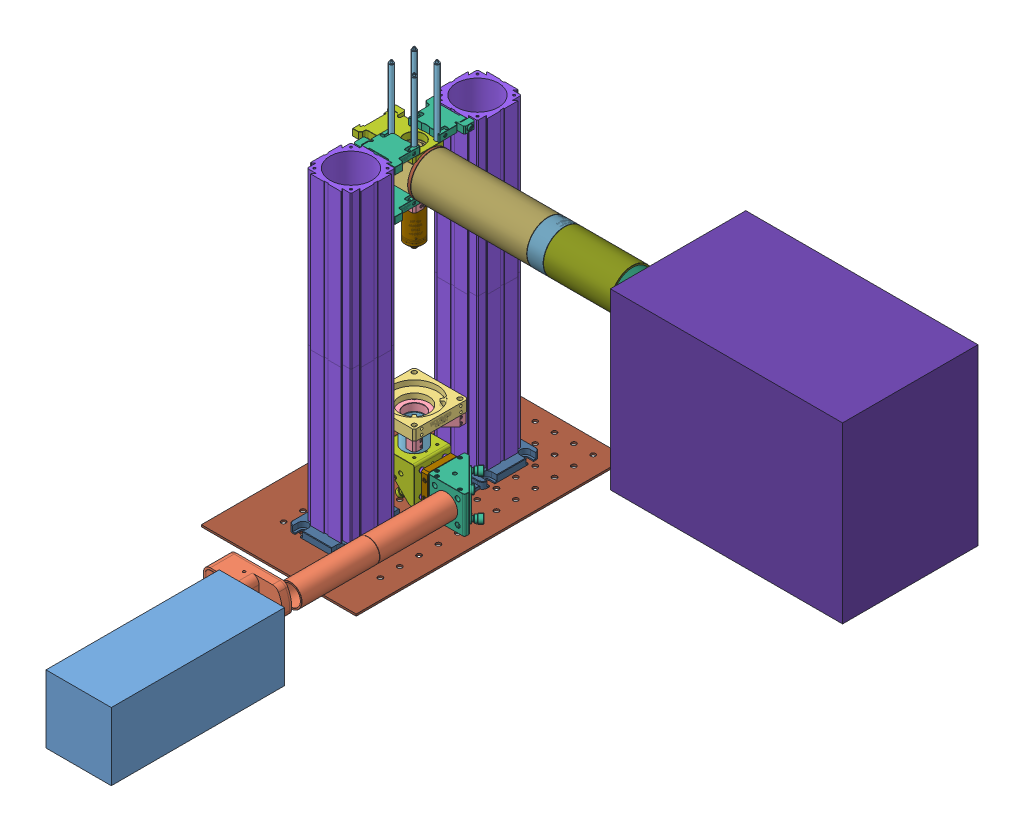
SolidWorks assembly Assembly, configuration Default. Lengths in mm.
Overall size (752.75 517.15 684.37).
51 component instances, 33 part files, 26 mates.
Components (placement in the parent):
- Laser-1: Laser [Default] at (-432.7153 -246.2224 392.8569) x (0 0 1) z (-1 0 0) size (238.02 88.9 85.74)
- SH05-Solidworks-1: SH05-Solidworks [Default] at (-478.4983 -151.3145 267.4556) x (0 1 0) z (0 0 -1) size (57.1 81.96 34.87)
- Objective Sub-Assembly-1: Objective Sub-Assembly [Default] at (-599.9053 226.5168 -25.2284) x (1 0 0) z (0 -1 0) size (97.86 248.79 490.2)
  - CM1-DCH-Solidworks-1: CM1-DCH-Solidworks [Web Assembly] at (101.1512 25.2284 74.1168) size (38.1 45.72 38.1)
  - CP16-Solidworks-1: CP16-Solidworks [Default] at (83.0447 27.4143 114.1512) size (41.22 40.64 8.89)
  - ER6-P4-Solidworks-1: ER6-P4-Solidworks [Default] at (115.9512 38.6905 31.8406) x (0.631657 -0.775248 0) z (-0.775248 -0.631657 0) size (5.99 157.48 5.99)
  - ER6-P4-Solidworks-2: ER6-P4-Solidworks [Default] at (114.7082 9.6603 31.8406) x (-0.373438 -0.927655 0) z (-0.927655 0.373438 0) size (5.99 157.48 5.99)
  - ER6-P4-Solidworks-3: ER6-P4-Solidworks [Default] at (85.1563 39.0388 31.8406) x (0.116187 -0.993227 0) z (-0.993227 -0.116187 0) size (5.99 157.48 5.99)
  - ER6-P4-Solidworks-4: ER6-P4-Solidworks [Default] at (87.3845 11.1687 36.8125) x (0.986967 -0.160923 0) z (0.160923 0.986967 0) size (5.99 157.48 5.99)
  - RCA2-Solidworks-1: RCA2-Solidworks [Default] at (87.6791 34.1856 4.2312) size (56.73 41.06 8.89)
  - RCA2-Solidworks-2: RCA2-Solidworks [Default] at (114.6233 16.2713 4.2312) x (-1 0 0) z (0 0 1) size (56.73 41.06 8.89)
  - RCA1-Solidworks-1: RCA1-Solidworks [Default] at (125.4438 -3.2318 -2.9001) x (0 1 0) z (0 0 1) size (56.5 73.55 8.89)
  - XT66-200-Solidworks-1: XT66-200-Solidworks [Default] at origin size (66.04 66.04 200)
  - XT66-200-Solidworks-2: XT66-200-Solidworks [Default] at (0 -166.04 0) size (66.04 66.04 200)
  - N40X-NIR-Solidworks-1: N40X-NIR-Solidworks [Default] at (101.1512 25.2284 137.1966) x (0 0 1) z (-0.615109 0.788442 0) size (61.98 27.94 27.94)
  - RCA2-Solidworks-3: RCA2-Solidworks [Default] at (114.6233 16.2713 60.4974) x (-1 0 0) z (0 0 1) size (56.73 41.06 8.89)
  - RCA2-Solidworks-4: RCA2-Solidworks [Default] at (87.6791 34.1856 60.4974) size (56.73 41.06 8.89)
  - XT66-200-Solidworks-3: XT66-200-Solidworks [Default] at (0 0 199.9996) size (66.04 66.04 200)
  - XT66-200-Solidworks-4: XT66-200-Solidworks [Default] at (0 -166.04 199.9996) size (66.04 66.04 200)
  - XT66P1-Solidworks-1: XT66P1-Solidworks [Default] at (101.1512 108.2611 445.7898) x (1 0 0) z (0 1 0) size (76.2 8.89 89.28)
  - XT66P1-Solidworks-2: XT66P1-Solidworks [Default] at (101.1385 -57.7916 445.7898) x (0 1 0) z (-1 0 0) size (76.2 8.89 89.28)
- Tank Sub-Assembly-1: Tank Sub-Assembly [Default] at origin size (492.39 222.91 245.75) (hidden)
  - WaterBath-1: WaterBath [Default] at (-614.8457 -4.3008 0) size (203.2 101.6 101.6)
  - L490-Solidworks-1: L490-Solidworks [Default] at (-624.5838 -100.8719 -9.0343) x (0 0 -1) z (1 0 0) size (245.75 83.31 101.6)
  - LX20-Solidworks-1: LX20-Solidworks [Chamfers] at (-650.9996 -116.3058 97.2581) size (132.4 38.28 116.16)
  - Opticell-1: Opticell [Default] at (-256.3578 52.6159 0) x (0.739747 0.672885 0) z (0 0 1) size (76.36 12.75 129.72)
- Camera Sub-Assembly-1: Camera Sub-Assembly [Default] at (-482.498 152.4 0) x (0 0.641515 0.767111) z (-1 0 0) size (71.93 71.93 328.57)
  - SM1A2-Solidworks-1: SM1A2-Solidworks [Default] at (0 0 -2.794) size (55.88 55.88 7.37)
  - SM2E60-Solidworks-1: SM2E60-Solidworks [Default] at (0 0 -83.312) x (-1 0 0) z (0 0 -1) size (55.88 55.88 155.45)
  - SM2NFM2-Solidworks-1: SM2NFM2-Solidworks [Default] at (0 0 -316.9027) x (0 1 0) z (-1 0 0) size (63.5 16.37 63.5)
  - TTL200-S8-Solidworks-1: TTL200-S8-Solidworks [Default] at (0 0 -170.337) size (55.88 55.88 28)
  - SM2V15-Solidworks-1: SM2V15-Solidworks [Default] at (18.0496 -29.8565 -319.6416) x (0 0 -1) z (0.951776 0.306793 0) size (51.56 57.15 57.15)
  - SM2M35-Solidworks-1: SM2M35-Solidworks [Default] at (-13.4416 4.8034 -237.3095) x (0.972414 0.233264 0) z (0 0 1) size (55.88 55.88 88.9)
- hpvx2-1: hpvx2 [Default] at origin size (311.15 228.6 177.8)
- Small Condenser Adjustable Sub-Assembly-1: Small Condenser Adjustable Sub-Assembly [Default] at (-430.8557 -214.193 -104.0018) x (0 -1 0) z (1 0 0) size (105.41 276.48 128.6)
  - LB1437-Solidworks-1: LB1437-Solidworks [Default] at (-24.13 -280.0439 -1.8596) x (0.911373 0 -0.411581) z (0 -1 0) size (25.4 25.4 3.05)
  - LB1761-Solidworks-1: LB1761-Solidworks [Default] at (-24.13 -135.2439 -1.8596) x (0.962182 0 -0.272406) z (0 -1 0) size (25.4 25.4 8.98)
  - SM1L40-Solidworks-1: SM1L40-Solidworks [Default] at (-22.2262 -175.3632 -3.9514) x (-1 0 0) z (0 1 0) size (30.48 30.48 105.41)
  - SM1L40-Solidworks-2: SM1L40-Solidworks [Default] at (-22.2262 -277.7252 -3.9514) x (-1 0 0) z (0 1 0) size (30.48 30.48 105.41)
  - CSA1003-Solidworks-1: CSA1003-Solidworks [Default] at (-52.7119 -190.8909 -81.6147) x (0 -1 0) z (0 0 1) size (71.12 13.97 71.12)
  - LCP02-Solidworks-1: LCP02-Solidworks [Default] at (-80.01 -104.0019 -67.8996) x (0 0 -1) z (1 0 0) size (70.75 70.61 12.7)
  - SM1S10-Solidworks-1: SM1S10-Solidworks [Default] at (-60.96 -104.0019 -67.8996) x (1 0 0) z (0 -0.505002 0.863118) size (31.5 30.48 30.48)
  - KCB1C-Solidworks-1: KCB1C-Solidworks [Default] at (-24.13 -104.0019 -1.8596) x (0 0 -1) z (0 -1 0) size (51.13 48.49 51.11)
  - KCB1-Solidworks-1: KCB1-Solidworks [Default] at (0 -79.8719 -92.0296) x (-1 0 0) z (0 0 1) size (51.13 48.26 51.1)
  - ER1-Solidworks-1: ER1-Solidworks [Default] at (-9.7751 -90.4123 -33.5555) x (0.374639 -0.927171 0) z (-0.927171 -0.374639 0) size (5.99 30.48 5.99)
  - ER1-Solidworks-2: ER1-Solidworks [Default] at (-9.1095 -120.5526 -33.5555) x (0.735372 -0.677663 0) z (-0.677663 -0.735372 0) size (5.99 30.48 5.99)
  - ER1-Solidworks-3: ER1-Solidworks [Default] at (-40.6715 -89.1711 -33.5555) x (-0.604001 -0.796983 0) z (-0.796983 0.604001 0) size (5.99 30.48 5.99)
  - ER1-Solidworks-4: ER1-Solidworks [Default] at (-40.6266 -118.5953 -33.5555) x (-0.853706 -0.520755 0) z (-0.520755 0.853706 0) size (5.99 30.48 5.99)
  - CP08-Solidworks-1: CP08-Solidworks [Default] at (-24.13 -104.002 -34.2446) x (0 1 0) z (0 0 1) size (41.5 40.64 8.89)
  - CPB1-Solidworks-1: CPB1-Solidworks [Default] at (5.08 -151.627 -27.2596) x (0 -1 0) z (0 0 -1) size (95.25 10.79 15.24)
- Table-1: Table [Default] at (-498.7541 -221.559 0) x (0 0 1) z (-1 0 0) size (355.6 2.54 203.2)
Mates (geometry in assembly coordinates):
- Concentric1: concentric anti-aligned: circle of Laser-1; circle of SH05-Solidworks-1
- Parallel1: parallel aligned: plane of Laser-1 through (-475.5856 -157.3224 279.1461) normal (-1 0 0); plane of SH05-Solidworks-1 through (-500.0253 -206.573 244.0941) normal (-1 0 0)
- Parallel2: parallel aligned: plane of Laser-1 through (0 -151.1382 0) normal (0 -1 0); plane of ? through (-543.2054 -139.4288 -36.195) normal (0 -1 0)
- Parallel3: parallel aligned: plane of Laser-1; plane of ? through (-458.1154 -135.6188 -46.99) normal (0 0 -1)
- Concentric2: concentric aligned: circle of SH05-Solidworks-1; circle of ?
- Parallel4: parallel aligned: plane of Laser-1 through (-432.7153 -246.2224 392.8569) normal (0 -1 0); plane of Objective Sub-Assembly-1/XT66-200-Solidworks-2 through (-469.6457 -10.3834 -100.4861) normal (0 -1 0)
- Concentric3: concentric anti-aligned: circle of ?; circle of Objective Sub-Assembly-1/RCA1-Solidworks-1
- Concentric4: concentric anti-aligned: circle of Objective Sub-Assembly-1/CM1-DCH-Solidworks-1; circle of Camera Sub-Assembly-1/SM1A2-Solidworks-1
- Coincident9: coincident anti-aligned: plane of Objective Sub-Assembly-1/CM1-DCH-Solidworks-1 through (-479.704 133.35 19.05) normal (1 0 0); plane of Camera Sub-Assembly-1/SM1A2-Solidworks-1 through (-479.704 173.8331 -17.9239) normal (-1 0 0)
- Concentric5: concentric anti-aligned: cylinder of Camera Sub-Assembly-1/SM2M35-Solidworks-1 through (-254.346 152.4 0) axis (-1 0 0) radius 27.94; cylinder of hpvx2-1 through (-152.4 152.4 0) axis (1 0 0) radius 29.1375
- Parallel9: parallel aligned: plane of Laser-1 through (-432.7153 -157.3224 392.8569) normal (0 1 0); plane of hpvx2-1 through (0 228.6 0) normal (0 1 0)
- Coincident10: coincident anti-aligned: plane of Camera Sub-Assembly-1/SM2NFM2-Solidworks-1 through (-158.75 152.4547 -0.0457) normal (1 0 0); plane of hpvx2-1 through (-158.75 152.4 0) normal (-1 0 0)
- Coincident13: coordinate: point of hpvx2-1; point of assembly
- Parallel10: parallel anti-aligned: plane of hpvx2-1 through (0 228.6 0) normal (0 1 0); plane of Small Condenser Adjustable Sub-Assembly-1/CPB1-Solidworks-1 through (-473.3553 -219.019 -28.5749) normal (0 -1 0)
- Parallel11: parallel aligned: plane of hpvx2-1 through (152.4 228.6 88.9) normal (1 0 0); plane of Small Condenser Adjustable Sub-Assembly-1/CSA1003-Solidworks-1 through (-463.1954 -113.863 -35.56) normal (1 0 0)
- Concentric6: concentric anti-aligned: circle of Objective Sub-Assembly-1/RCA1-Solidworks-1; circle of Small Condenser Adjustable Sub-Assembly-1/CSA1003-Solidworks-1
- Concentric7: concentric anti-aligned: circle of Laser-1; circle of Small Condenser Adjustable Sub-Assembly-1/SM1L40-Solidworks-2
- Distance5: distance = 25.4 mm anti-aligned: plane of SH05-Solidworks-1 through (-462.8502 -190.2676 253.7461) normal (0 0 1); plane of Laser-1 through (-475.5856 -157.3224 279.1461) normal (0 0 -1)
- Distance6: distance = 12.7 mm anti-aligned: plane of SH05-Solidworks-1 through (-462.8502 -190.2676 241.5541) normal (0 0 -1); plane of Small Condenser Adjustable Sub-Assembly-1/SM1L40-Solidworks-2 through (-417.7293 -190.063 228.8541) normal (0 0 1)
- Parallel12: parallel anti-aligned: plane of hpvx2-1 through (152.4 228.6 88.9) normal (1 0 0); plane of Table-1 through (-600.3541 -219.019 -177.8) normal (-1 0 0)
- Coincident19: coincident aligned: plane of Table-1 through (-498.7541 -221.559 0) normal (0 0 1); plane of assembly through (0 0 0) normal (0 0 1)
- Coincident20: coincident aligned: plane of Objective Sub-Assembly-1/XT66-200-Solidworks-1 through (-498.7541 226.5168 -25.2284) normal (-1 0 0); plane of Table-1 through (-498.7541 -221.559 0) normal (-1 0 0)
- Coincident21: coincident anti-aligned: plane of Objective Sub-Assembly-1/XT66P1-Solidworks-1 through (-482.8791 -219.019 98.9077) normal (0 -1 0); plane of Table-1 through (-498.7541 -219.019 0) normal (0 1 0)
- Coincident22: coincident anti-aligned: plane of Small Condenser Adjustable Sub-Assembly-1/CPB1-Solidworks-1 through (-473.3553 -219.019 -28.5749) normal (0 -1 0); plane of Table-1 through (-498.7541 -219.019 0) normal (0 1 0)
- Coincident23: coincident aligned: plane of Tank Sub-Assembly-1/WaterBath-1 through (-614.8457 -4.3008 0) normal (0 0 1); plane of assembly through (0 0 0) normal (0 0 1)
- Parallel13: parallel aligned: plane of Laser-1 through (-432.7153 -157.3224 392.8569) normal (0 1 0); plane of Tank Sub-Assembly-1/L490-Solidworks-1 through (-564.0457 -4.3008 -50.8) normal (0 1 0)
